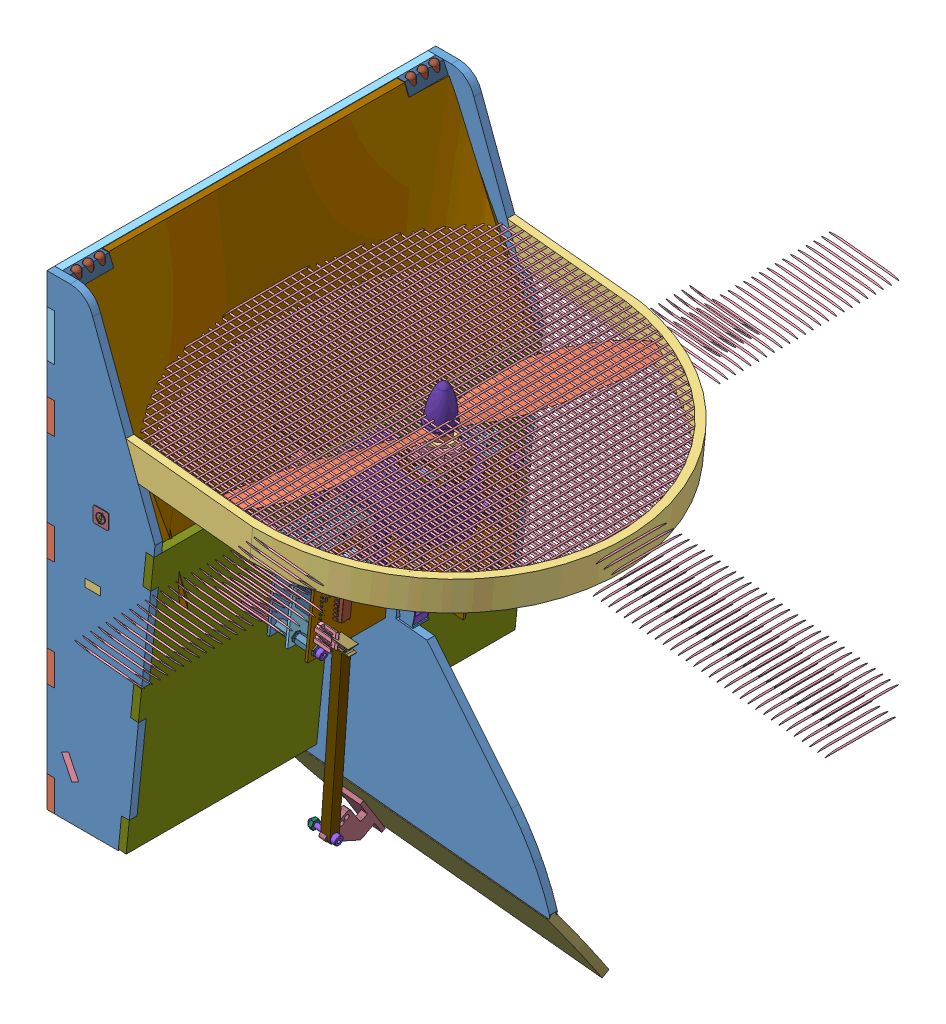
SolidWorks assembly AssTotaleSimu6, configuration Défaut. Lengths in mm.
Overall size (253.25 382.9 251.6).
1779 component instances, 238 part files, 11 mates.
Components (placement in the parent):
- AssStructSimu-1: AssStructSimu [Défaut] at (-125.7658 -1.8483 624.6548) x (1 0 0) z (0 0 -1) size (253.25 324.59 251.6)
  - AssBase-1: AssBase [Défaut] at (36.5482 -71.0398 34.0612) size (86.08 302.3 251.6)
    - AssD-1: AssD [Défaut] at (39.0992 31.0201 8.5) size (69.5 300 22)
      - P1-1: P1 [Défaut] at (-95.5819 194.6656 377.5) size (69.5 300 5)
      - P5-1: P5 [Défaut] at (-100.5819 -35.3344 360.5) x (0 1 0) z (1 0 0) size (230 22 5)
    - AssG-1: AssG [Défaut] at (39.0992 31.0201 -236.5) size (69.5 300 22)
      - P1-1: P1 [Défaut] at (-95.5819 194.6656 377.5) size (69.5 300 5)
      - P5-1: P5 [Défaut] at (-95.5819 -35.3344 399.5) x (0 1 0) z (-1 0 0) size (230 22 5)
    - P7-1: P7 [Défaut] at (-1.4828 89.6857 370.5) x (0 0 -1) z (0 -1 0) size (250 54.5 5)
    - P4-1: P4 [Défaut] at (-63.2363 165.9323 386) x (0 0 -1) z (0.898794 -0.438371 0) size (250 60.5 66.27)
    - P3-1: P3 [Défaut] at (-56.4828 -74.3143 146) x (0 0 1) z (-1 0 0) size (250 70 5)
    - P4b-1: P4b [Défaut] at (-58.7423 163.7404 190) x (0 0 1) z (0.438371 0.898794 0) size (152 56 2)
    - battery-1: battery [Défaut] at (-39.0156 204.1861 197.5) x (0 0 1) z (0.898794 -0.438371 0) size (137 43 30)
    - socket head cap screw 4762_din-1: socket head cap screw 4762_din [EN ISO 4762 M3 x 10 - 10N] at (-27.7008 145.2627 193) x (0.438371 0.898794 0) z (0 0 -1) size (13 5.5 5.5)
    - socket head cap screw 4762_din-2: socket head cap screw 4762_din [EN ISO 4762 M3 x 10 - 10N] at (-27.7008 145.2627 339) x (0.438371 0.898794 0) z (-0.791285 0.385936 -0.474259) size (13 5.5 5.5)
    - socket head cap screw 4762_din-3: socket head cap screw 4762_din [EN ISO 4762 M3 x 10 - 10N] at (-42.0815 152.2766 339) x (0.438371 0.898794 0) z (-0.001489 0.000726 -0.999999) size (13 5.5 5.5)
    - socket head cap screw 4762_din-4: socket head cap screw 4762_din [EN ISO 4762 M3 x 10 - 10N] at (-42.0815 152.2766 193) x (0.438371 0.898794 0) z (-0.031331 0.015281 -0.999392) size (13 5.5 5.5)
    - P11-1: P11 [Défaut] at (-57.5734 -73.9703 146.7843) x (0.005072 0 0.999987) z (0.006197 0.999981 -0.000031) size (240 65 164)
    - AssPhare-1: AssPhare [Défaut] at (-52.8518 -67.6977 411) x (0 1 0) z (0 0 -1) size (35.8 8 25)
      - piece_led-1: piece_led [Défaut] at (-6.6166 -3.631 25) size (7 8 25)
      - LED 5mm-1: LED 5mm [Valor predeterminado] at (-0.1166 0.369 30) x (0 0 1) z (-1 0 0) size (10.06 6 40.8)
      - LED 5mm-2: LED 5mm [Valor predeterminado] at (-0.1166 0.369 37.5) x (0 0 1) z (-1 0 0) size (10.06 6 40.8)
      - LED 5mm-3: LED 5mm [Valor predeterminado] at (-0.1166 0.369 45) x (0 0 1) z (-1 0 0) size (10.06 6 40.8)
    - AssPhare-2: AssPhare [Défaut] at (-52.8518 -67.6977 196) x (0 1 0) z (0 0 -1) size (35.8 8 25)
      - piece_led-1: piece_led [Défaut] at (-6.6166 -3.631 25) size (7 8 25)
      - LED 5mm-1: LED 5mm [Valor predeterminado] at (-0.1166 0.369 30) x (0 0 1) z (-1 0 0) size (10.06 6 40.8)
      - LED 5mm-2: LED 5mm [Valor predeterminado] at (-0.1166 0.369 37.5) x (0 0 1) z (-1 0 0) size (10.06 6 40.8)
      - LED 5mm-3: LED 5mm [Valor predeterminado] at (-0.1166 0.369 45) x (0 0 1) z (-1 0 0) size (10.06 6 40.8)
    - AssLogo-1: AssLogo [Défaut] at (-27.8835 45.1673 148.1054) x (-1 0 0) z (0 0 -1) size (10 10 0.8)
      - logo1-1: logo1 [Défaut] at (-6.5271 -4.4734 6.5054) size (5.8 7.71 0.4)
      - logo2-1: logo2 [Défaut] at (-6.4007 -4.4815 7.1054) size (10 10 0.4)
    - AssLogo-2: AssLogo [Défaut] at (-25.082 45.1673 383.8946) size (10 10 0.8)
      - logo1-1: logo1 [Défaut] at (-6.5271 -4.4734 6.5054) size (5.8 7.71 0.4)
      - logo2-1: logo2 [Défaut] at (-6.4007 -4.4815 7.1054) size (10 10 0.4)
    - support2-1: support2 [Défaut] at (-61.5648 191.7124 276) x (-0.017452 -0.999848 0) z (0.999848 -0.017452 0) size (75 20 10)
    - socket head cap screw 4762_din-5: socket head cap screw 4762_din [EN ISO 4762 M3 x 5 - 5N] at (-61.652 186.7132 269.3333) x (0.999848 -0.017452 0) z (-0.002158 -0.123615 0.992328) size (8 5.5 5.5)
    - socket head cap screw 4762_din-6: socket head cap screw 4762_din [EN ISO 4762 M3 x 5 - 5N] at (-61.652 186.7132 262.6667) x (0.999848 -0.017452 0) z (0 0 1) size (8 5.5 5.5)
    - socket head cap screw 4762_din-7: socket head cap screw 4762_din [EN ISO 4762 M3 x 25 - 18N] at (-55.2963 121.0922 253) x (0 0 1) z (-1 0 0) size (28 5.5 5.5)
    - hex nut style 1 gradeab_din-1: hex nut style 1 gradeab_din [Hexagon Nut ISO 4032 - M3 - W - N] at (-55.2963 121.0922 276) x (-0.923728 -0.383049 0) z (0 0 -1) size (5.5 6.35 2.4)
  - AssToitMot-1: AssToitMot [Défaut] at (-168.5238 43.6961 238.494) x (0 0 -1) z (0.9948 0.101852 0) size (250 207.5 205)
    - AssToit-1: AssToit [Défaut] at (-23.0702 -16.5789 -3.7148) size (250 207.5 205)
      - P8-1: P8 [Défaut] at (-38.4971 122.5921 203.5) size (250 175 5)
      - P12-1: P12 [Défaut] at (-60.4971 -63.4079 265.5) x (1 0 0) z (0 -1 0) size (44.28 76.64 55)
      - P13-1: P13 [Défaut] at (-35.9971 -52.8579 208.5) x (0 0 1) z (-1 0 0) size (64 15.55 5)
      - P10_2-1: P10_2 [Défaut] at (-35.9971 111.5921 171) x (0 0 1) z (-1 0 0) size (188.5 117.6 5)
    - Parallax-Servo_DUMMY-1: Parallax-Servo_DUMMY [Défaut] at (-61.6002 -51.5207 216.6662) x (1 0 0) z (0 1 0) size (20.07 42.67 55.64)
    - socket head cap screw 4762_din-1: socket head cap screw 4762_din [EN ISO 4762 M2.5 x 5 - 5N] at (-51.9272 -76.4868 259.2852) x (0 -1 0) z (-0.546944 0 0.837169) size (7.5 4.5 4.5)
    - socket head cap screw 4762_din-2: socket head cap screw 4762_din [EN ISO 4762 M2.5 x 5 - 5N] at (-61.5672 -76.4868 268.9252) x (0 -1 0) z (-0.546944 0 0.837169) size (7.5 4.5 4.5)
    - socket head cap screw 4762_din-3: socket head cap screw 4762_din [EN ISO 4762 M2.5 x 5 - 5N] at (-71.2072 -76.4868 259.2852) x (0 -1 0) z (-0.546944 0 0.837169) size (7.5 4.5 4.5)
    - socket head cap screw 4762_din-4: socket head cap screw 4762_din [EN ISO 4762 M2.5 x 5 - 5N] at (-61.5672 -76.4868 249.6452) x (0 -1 0) z (-0.546944 0 0.837169) size (7.5 4.5 4.5)
    - AssPhare-1: AssPhare [Défaut] at (8.4328 83.3966 196.1542) x (0 -1 0) z (1 0 0) size (35.8 8 25)
      - piece_led-1: piece_led [Défaut] at (-6.6166 -3.631 25) size (7 8 25)
      - LED 5mm-1: LED 5mm [Valor predeterminado] at (-0.1166 0.369 30) x (0 0 1) z (-1 0 0) size (10.06 6 40.8)
      - LED 5mm-2: LED 5mm [Valor predeterminado] at (-0.1166 0.369 37.5) x (0 0 1) z (-1 0 0) size (10.06 6 40.8)
      - LED 5mm-3: LED 5mm [Valor predeterminado] at (-0.1166 0.369 45) x (0 0 1) z (-1 0 0) size (10.06 6 40.8)
    - AssPhare-2: AssPhare [Défaut] at (-206.5672 83.3966 196.1542) x (0 -1 0) z (1 0 0) size (35.8 8 25)
      - piece_led-1: piece_led [Défaut] at (-6.6166 -3.631 25) size (7 8 25)
      - LED 5mm-1: LED 5mm [Valor predeterminado] at (-0.1166 0.369 30) x (0 0 1) z (-1 0 0) size (10.06 6 40.8)
      - LED 5mm-2: LED 5mm [Valor predeterminado] at (-0.1166 0.369 37.5) x (0 0 1) z (-1 0 0) size (10.06 6 40.8)
      - LED 5mm-3: LED 5mm [Valor predeterminado] at (-0.1166 0.369 45) x (0 0 1) z (-1 0 0) size (10.06 6 40.8)
    - socket head cap screw 4762_din-5: socket head cap screw 4762_din [EN ISO 4762 M3 x 10 - 10N] at (-67.0672 -22.9368 210.2852) x (0 0 -1) z (1 0 0) size (13 5.5 5.5)
    - socket head cap screw 4762_din-6: socket head cap screw 4762_din [EN ISO 4762 M3 x 10 - 10N] at (-56.0672 -72.9868 210.2852) x (0 0 -1) z (1 0 0) size (13 5.5 5.5)
    - socket head cap screw 4762_din-7: socket head cap screw 4762_din [EN ISO 4762 M3 x 10 - 10N] at (-67.0672 -72.9868 210.2852) x (0 0 -1) z (1 0 0) size (13 5.5 5.5)
    - socket head cap screw 4762_din-8: socket head cap screw 4762_din [EN ISO 4762 M3 x 10 - 10N] at (-56.0672 -22.9368 210.2852) x (0 0 -1) z (1 0 0) size (13 5.5 5.5)
    - hex nut style 1 gradeab_din-1: hex nut style 1 gradeab_din [Hexagon Nut ISO 4032 - M3 - W - N] at (-67.0672 -72.9868 197.3852) x (-0.923728 -0.383049 0) z (0 0 -1) size (5.5 6.35 2.4)
    - hex nut style 1 gradeab_din-2: hex nut style 1 gradeab_din [Hexagon Nut ISO 4032 - M3 - W - N] at (-56.0672 -72.9868 199.7852) size (5.5 6.35 2.4)
    - hex nut style 1 gradeab_din-3: hex nut style 1 gradeab_din [Hexagon Nut ISO 4032 - M3 - W - N] at (-67.0672 -22.9368 199.7852) size (5.5 6.35 2.4)
    - hex nut style 1 gradeab_din-4: hex nut style 1 gradeab_din [Hexagon Nut ISO 4032 - M3 - W - N] at (-56.0672 -22.9368 199.7852) size (5.5 6.35 2.4)
  - AssProtec-1: AssProtec [Défaut] at (86.6746 190.4649 284.6351) x (0 0 -1) z (0.101852 -0.9948 0) size (250 237.46 20)
    - protec3c-1: protec3c [Défaut] at (-140.4261 -87.7568 240) size (250 197 20)
    - AssGrillage-1: AssGrillage [Défaut] at (-370.4609 -132.5428 258.3161) x (0 0 -1) z (1 0 0) size (2.02 237.05 250)
      - barreau-1: barreau [Défaut] at (-1.1839 0.254 200) size (1 1 400)
      - barreau-3: barreau [Défaut] at (-1.1839 5.254 200) size (1 1 400)
      - barreau-4: barreau [Défaut] at (-1.1839 10.254 200) size (1 1 400)
      - barreau-5: barreau [Défaut] at (-1.1839 15.254 200) size (1 1 400)
      - barreau-6: barreau [Défaut] at (-1.1839 20.254 200) size (1 1 400)
      - barreau-7: barreau [Défaut] at (-1.1839 25.254 200) size (1 1 400)
      - barreau-8: barreau [Défaut] at (-1.1839 30.254 200) size (1 1 400)
      - barreau-9: barreau [Défaut] at (-1.1839 35.254 200) size (1 1 400)
      - barreau-10: barreau [Défaut] at (-1.1839 40.254 200) size (1 1 400)
      - barreau-11: barreau [Défaut] at (-1.1839 45.254 200) size (1 1 400)
      - barreau-12: barreau [Défaut] at (-1.1839 50.254 200) size (1 1 400)
      - barreau-13: barreau [Défaut] at (-1.1839 55.254 200) size (1 1 400)
      - barreau-14: barreau [Défaut] at (-1.1839 60.254 200) size (1 1 400)
      - barreau-15: barreau [Défaut] at (-1.1839 65.254 200) size (1 1 400)
      - barreau-16: barreau [Défaut] at (-1.1839 70.254 200) size (1 1 400)
      - barreau-17: barreau [Défaut] at (-1.1839 75.254 200) size (1 1 400)
      - barreau-18: barreau [Défaut] at (-1.1839 80.254 200) size (1 1 400)
      - barreau-19: barreau [Défaut] at (-1.1839 85.254 200) size (1 1 400)
      - barreau-20: barreau [Défaut] at (-1.1839 90.254 200) size (1 1 400)
      - barreau-21: barreau [Défaut] at (-1.1839 95.254 200) size (1 1 400)
      - barreau-22: barreau [Défaut] at (-1.1839 100.254 200) size (1 1 400)
      - barreau-23: barreau [Défaut] at (-1.1839 105.254 200) size (1 1 400)
      - barreau-24: barreau [Défaut] at (-1.1839 110.254 200) size (1 1 400)
      - barreau-25: barreau [Défaut] at (-1.1839 115.254 200) size (1 1 400)
      - barreau-26: barreau [Défaut] at (-1.1839 120.254 200) size (1 1 400)
      - barreau-27: barreau [Défaut] at (-1.1839 125.254 200) size (1 1 400)
      - barreau-28: barreau [Défaut] at (-1.1839 130.254 200) size (1 1 400)
      - barreau-29: barreau [Défaut] at (-1.1839 135.254 200) size (1 1 400)
      - barreau-30: barreau [Défaut] at (-1.1839 140.254 200) size (1 1 400)
      - barreau-31: barreau [Défaut] at (-1.1839 145.254 200) size (1 1 400)
      - barreau-32: barreau [Défaut] at (-1.1839 150.254 200) size (1 1 400)
      - barreau-33: barreau [Défaut] at (-1.1839 155.254 200) size (1 1 400)
      - barreau-34: barreau [Défaut] at (-1.1839 160.254 200) size (1 1 400)
      - barreau-35: barreau [Défaut] at (-1.1839 165.254 200) size (1 1 400)
      - barreau-36: barreau [Défaut] at (-1.1839 170.254 200) size (1 1 400)
      - barreau-37: barreau [Défaut] at (-1.1839 175.254 200) size (1 1 400)
      - barreau-38: barreau [Défaut] at (-1.1839 180.254 200) size (1 1 400)
      - barreau-39: barreau [Défaut] at (-1.1839 185.254 200) size (1 1 400)
      - barreau-40: barreau [Défaut] at (-1.1839 190.254 200) size (1 1 400)
      - barreau-41: barreau [Défaut] at (-1.1839 195.254 200) size (1 1 400)
      - barreau-42: barreau [Défaut] at (-0.1839 -1.5314 598.7823) x (0.998922 0 0.04641) z (0 1 0) size (1 1 400)
      - barreau-43: barreau [Défaut] at (-1.1839 200.254 200) size (1 1 400)
      - barreau-44: barreau [Défaut] at (-1.1839 205.254 200) size (1 1 400)
      - barreau-45: barreau [Défaut] at (-1.1839 210.254 200) size (1 1 400)
      - barreau-46: barreau [Défaut] at (-1.1839 215.254 200) size (1 1 400)
      - barreau-47: barreau [Défaut] at (-1.1839 220.254 200) size (1 1 400)
      - barreau-48: barreau [Défaut] at (-1.1839 225.254 200) size (1 1 400)
      - barreau-49: barreau [Défaut] at (-1.1839 230.254 200) size (1 1 400)
      - barreau-50: barreau [Défaut] at (-1.1839 235.254 200) size (1 1 400)
      - barreau-51: barreau [Défaut] at (-1.1839 240.254 200) size (1 1 400)
      - barreau-52: barreau [Défaut] at (-1.1839 245.254 200) size (1 1 400)
      - barreau-53: barreau [Défaut] at (-1.1839 250.254 200) size (1 1 400)
      - barreau-54: barreau [Défaut] at (-1.1839 255.254 200) size (1 1 400)
      - barreau-55: barreau [Défaut] at (-1.1839 260.254 200) size (1 1 400)
      - barreau-56: barreau [Défaut] at (-1.1839 265.254 200) size (1 1 400)
      - barreau-57: barreau [Défaut] at (-1.1839 270.254 200) size (1 1 400)
      - barreau-58: barreau [Défaut] at (-1.1839 275.254 200) size (1 1 400)
      - barreau-59: barreau [Défaut] at (-1.1839 280.254 200) size (1 1 400)
      - barreau-60: barreau [Défaut] at (-1.1839 285.254 200) size (1 1 400)
      - barreau-61: barreau [Défaut] at (-1.1839 290.254 200) size (1 1 400)
      - barreau-62: barreau [Défaut] at (-1.1839 295.254 200) size (1 1 400)
      - barreau-63: barreau [Défaut] at (-1.1839 300.254 200) size (1 1 400)
      - barreau-64: barreau [Défaut] at (-1.1839 305.254 200) size (1 1 400)
      - barreau-65: barreau [Défaut] at (-1.1839 310.254 200) size (1 1 400)
      - barreau-66: barreau [Défaut] at (-1.1839 315.254 200) size (1 1 400)
      - barreau-67: barreau [Défaut] at (-1.1839 320.254 200) size (1 1 400)
      - barreau-68: barreau [Défaut] at (-1.1839 325.254 200) size (1 1 400)
      - barreau-69: barreau [Défaut] at (-1.1839 330.254 200) size (1 1 400)
      - barreau-70: barreau [Défaut] at (-1.1839 335.254 200) size (1 1 400)
      - barreau-71: barreau [Défaut] at (-1.1839 340.254 200) size (1 1 400)
      - barreau-72: barreau [Défaut] at (-1.1839 345.254 200) size (1 1 400)
      - barreau-73: barreau [Défaut] at (-1.1839 350.254 200) size (1 1 400)
      - barreau-74: barreau [Défaut] at (-1.1839 355.254 200) size (1 1 400)
      - barreau-75: barreau [Défaut] at (-1.1839 360.254 200) size (1 1 400)
      - barreau-76: barreau [Défaut] at (-1.1839 365.254 200) size (1 1 400)
      - barreau-77: barreau [Défaut] at (-1.1839 370.254 200) size (1 1 400)
      - barreau-78: barreau [Défaut] at (-1.1839 375.254 200) size (1 1 400)
      - barreau-79: barreau [Défaut] at (-1.1839 380.254 200) size (1 1 400)
      - barreau-80: barreau [Défaut] at (-1.1839 385.254 200) size (1 1 400)
      - barreau-81: barreau [Défaut] at (-1.1839 390.254 200) size (1 1 400)
      - barreau-82: barreau [Défaut] at (-1.1839 395.254 200) size (1 1 400)
      - barreau-136: barreau [Défaut] at (-0.1839 -1.5314 593.7823) x (0.998922 0 0.04641) z (0 1 0) size (1 1 400)
      - barreau-137: barreau [Défaut] at (-0.1839 -1.5314 588.7823) x (0.998922 0 0.04641) z (0 1 0) size (1 1 400)
      - barreau-138: barreau [Défaut] at (-0.1839 -1.5314 583.7823) x (0.998922 0 0.04641) z (0 1 0) size (1 1 400)
      - barreau-139: barreau [Défaut] at (-0.1839 -1.5314 578.7823) x (0.998922 0 0.04641) z (0 1 0) size (1 1 400)
      - barreau-140: barreau [Défaut] at (-0.1839 -1.5314 573.7823) x (0.998922 0 0.04641) z (0 1 0) size (1 1 400)
      - barreau-141: barreau [Défaut] at (-0.1839 -1.5314 568.7823) x (0.998922 0 0.04641) z (0 1 0) size (1 1 400)
      - barreau-142: barreau [Défaut] at (-0.1839 -1.5314 563.7823) x (0.998922 0 0.04641) z (0 1 0) size (1 1 400)
      - barreau-143: barreau [Défaut] at (-0.1839 -1.5314 558.7823) x (0.998922 0 0.04641) z (0 1 0) size (1 1 400)
      - barreau-144: barreau [Défaut] at (-0.1839 -1.5314 553.7823) x (0.998922 0 0.04641) z (0 1 0) size (1 1 400)
      - barreau-145: barreau [Défaut] at (-0.1839 -1.5314 548.7823) x (0.998922 0 0.04641) z (0 1 0) size (1 1 400)
      - barreau-146: barreau [Défaut] at (-0.1839 -1.5314 543.7823) x (0.998922 0 0.04641) z (0 1 0) size (1 1 400)
      - barreau-147: barreau [Défaut] at (-0.1839 -1.5314 538.7823) x (0.998922 0 0.04641) z (0 1 0) size (1 1 400)
      - barreau-148: barreau [Défaut] at (-0.1839 -1.5314 533.7823) x (0.998922 0 0.04641) z (0 1 0) size (1 1 400)
      - barreau-149: barreau [Défaut] at (-0.1839 -1.5314 528.7823) x (0.998922 0 0.04641) z (0 1 0) size (1 1 400)
      - barreau-150: barreau [Défaut] at (-0.1839 -1.5314 523.7823) x (0.998922 0 0.04641) z (0 1 0) size (1 1 400)
      - barreau-151: barreau [Défaut] at (-0.1839 -1.5314 518.7823) x (0.998922 0 0.04641) z (0 1 0) size (1 1 400)
      - barreau-152: barreau [Défaut] at (-0.1839 -1.5314 513.7823) x (0.998922 0 0.04641) z (0 1 0) size (1 1 400)
      - barreau-153: barreau [Défaut] at (-0.1839 -1.5314 508.7823) x (0.998922 0 0.04641) z (0 1 0) size (1 1 400)
      - barreau-154: barreau [Défaut] at (-0.1839 -1.5314 503.7823) x (0.998922 0 0.04641) z (0 1 0) size (1 1 400)
      - barreau-155: barreau [Défaut] at (-0.1839 -1.5314 498.7823) x (0.998922 0 0.04641) z (0 1 0) size (1 1 400)
      - barreau-156: barreau [Défaut] at (-0.1839 -1.5314 493.7823) x (0.998922 0 0.04641) z (0 1 0) size (1 1 400)
      - barreau-157: barreau [Défaut] at (-0.1839 -1.5314 488.7823) x (0.998922 0 0.04641) z (0 1 0) size (1 1 400)
      - barreau-158: barreau [Défaut] at (-0.1839 -1.5314 483.7823) x (0.998922 0 0.04641) z (0 1 0) size (1 1 400)
      - barreau-159: barreau [Défaut] at (-0.1839 -1.5314 478.7823) x (0.998922 0 0.04641) z (0 1 0) size (1 1 400)
      - barreau-160: barreau [Défaut] at (-0.1839 -1.5314 473.7823) x (0.998922 0 0.04641) z (0 1 0) size (1 1 400)
      - barreau-161: barreau [Défaut] at (-0.1839 -1.5314 468.7823) x (0.998922 0 0.04641) z (0 1 0) size (1 1 400)
      - barreau-162: barreau [Défaut] at (-0.1839 -1.5314 463.7823) x (0.998922 0 0.04641) z (0 1 0) size (1 1 400)
      - barreau-163: barreau [Défaut] at (-0.1839 -1.5314 458.7823) x (0.998922 0 0.04641) z (0 1 0) size (1 1 400)
      - barreau-164: barreau [Défaut] at (-0.1839 -1.5314 453.7823) x (0.998922 0 0.04641) z (0 1 0) size (1 1 400)
      - barreau-165: barreau [Défaut] at (-0.1839 -1.5314 448.7823) x (0.998922 0 0.04641) z (0 1 0) size (1 1 400)
      - barreau-166: barreau [Défaut] at (-0.1839 -1.5314 443.7823) x (0.998922 0 0.04641) z (0 1 0) size (1 1 400)
      - barreau-167: barreau [Défaut] at (-0.1839 -1.5314 438.7823) x (0.998922 0 0.04641) z (0 1 0) size (1 1 400)
      - barreau-168: barreau [Défaut] at (-0.1839 -1.5314 433.7823) x (0.998922 0 0.04641) z (0 1 0) size (1 1 400)
      - barreau-169: barreau [Défaut] at (-0.1839 -1.5314 428.7823) x (0.998922 0 0.04641) z (0 1 0) size (1 1 400)
      - barreau-170: barreau [Défaut] at (-0.1839 -1.5314 423.7823) x (0.998922 0 0.04641) z (0 1 0) size (1 1 400)
      - barreau-171: barreau [Défaut] at (-0.1839 -1.5314 418.7823) x (0.998922 0 0.04641) z (0 1 0) size (1 1 400)
      - barreau-172: barreau [Défaut] at (-0.1839 -1.5314 413.7823) x (0.998922 0 0.04641) z (0 1 0) size (1 1 400)
      - barreau-173: barreau [Défaut] at (-0.1839 -1.5314 408.7823) x (0.998922 0 0.04641) z (0 1 0) size (1 1 400)
      - barreau-174: barreau [Défaut] at (-0.1839 -1.5314 403.7823) x (0.998922 0 0.04641) z (0 1 0) size (1 1 400)
      - barreau-175: barreau [Défaut] at (-0.1839 -1.5314 398.7823) x (0.998922 0 0.04641) z (0 1 0) size (1 1 400)
      - barreau-176: barreau [Défaut] at (-0.1839 -1.5314 393.7823) x (0.998922 0 0.04641) z (0 1 0) size (1 1 400)
      - barreau-177: barreau [Défaut] at (-0.1839 -1.5314 388.7823) x (0.998922 0 0.04641) z (0 1 0) size (1 1 400)
      - barreau-178: barreau [Défaut] at (-0.1839 -1.5314 383.7823) x (0.998922 0 0.04641) z (0 1 0) size (1 1 400)
      - barreau-179: barreau [Défaut] at (-0.1839 -1.5314 378.7823) x (0.998922 0 0.04641) z (0 1 0) size (1 1 400)
      - barreau-180: barreau [Défaut] at (-0.1839 -1.5314 373.7823) x (0.998922 0 0.04641) z (0 1 0) size (1 1 400)
      - barreau-181: barreau [Défaut] at (-0.1839 -1.5314 368.7823) x (0.998922 0 0.04641) z (0 1 0) size (1 1 400)
      - barreau-182: barreau [Défaut] at (-0.1839 -1.5314 363.7823) x (0.998922 0 0.04641) z (0 1 0) size (1 1 400)
      - barreau-183: barreau [Défaut] at (-0.1839 -1.5314 358.7823) x (0.998922 0 0.04641) z (0 1 0) size (1 1 400)
      - barreau-184: barreau [Défaut] at (-0.1839 -1.5314 353.7823) x (0.998922 0 0.04641) z (0 1 0) size (1 1 400)
      - barreau-185: barreau [Défaut] at (-0.1839 -1.5314 348.7823) x (0.998922 0 0.04641) z (0 1 0) size (1 1 400)
      - barreau-186: barreau [Défaut] at (-0.1839 -1.5314 343.7823) x (0.998922 0 0.04641) z (0 1 0) size (1 1 400)
      - barreau-187: barreau [Défaut] at (-0.1839 -1.5314 338.7823) x (0.998922 0 0.04641) z (0 1 0) size (1 1 400)
      - barreau-188: barreau [Défaut] at (-0.1839 -1.5314 333.7823) x (0.998922 0 0.04641) z (0 1 0) size (1 1 400)
      - barreau-189: barreau [Défaut] at (-0.1839 -1.5314 328.7823) x (0.998922 0 0.04641) z (0 1 0) size (1 1 400)
      - barreau-190: barreau [Défaut] at (-0.1839 -1.5314 323.7823) x (0.998922 0 0.04641) z (0 1 0) size (1 1 400)
      - barreau-191: barreau [Défaut] at (-0.1839 -1.5314 318.7823) x (0.998922 0 0.04641) z (0 1 0) size (1 1 400)
      - barreau-192: barreau [Défaut] at (-0.1839 -1.5314 313.7823) x (0.998922 0 0.04641) z (0 1 0) size (1 1 400)
      - barreau-193: barreau [Défaut] at (-0.1839 -1.5314 308.7823) x (0.998922 0 0.04641) z (0 1 0) size (1 1 400)
      - barreau-194: barreau [Défaut] at (-0.1839 -1.5314 303.7823) x (0.998922 0 0.04641) z (0 1 0) size (1 1 400)
      - barreau-195: barreau [Défaut] at (-0.1839 -1.5314 298.7823) x (0.998922 0 0.04641) z (0 1 0) size (1 1 400)
      - barreau-196: barreau [Défaut] at (-0.1839 -1.5314 293.7823) x (0.998922 0 0.04641) z (0 1 0) size (1 1 400)
      - barreau-197: barreau [Défaut] at (-0.1839 -1.5314 288.7823) x (0.998922 0 0.04641) z (0 1 0) size (1 1 400)
      - barreau-198: barreau [Défaut] at (-0.1839 -1.5314 283.7823) x (0.998922 0 0.04641) z (0 1 0) size (1 1 400)
      - barreau-199: barreau [Défaut] at (-0.1839 -1.5314 278.7823) x (0.998922 0 0.04641) z (0 1 0) size (1 1 400)
      - barreau-200: barreau [Défaut] at (-0.1839 -1.5314 273.7823) x (0.998922 0 0.04641) z (0 1 0) size (1 1 400)
      - barreau-201: barreau [Défaut] at (-0.1839 -1.5314 268.7823) x (0.998922 0 0.04641) z (0 1 0) size (1 1 400)
      - barreau-202: barreau [Défaut] at (-0.1839 -1.5314 263.7823) x (0.998922 0 0.04641) z (0 1 0) size (1 1 400)
      - barreau-203: barreau [Défaut] at (-0.1839 -1.5314 258.7823) x (0.998922 0 0.04641) z (0 1 0) size (1 1 400)
      - barreau-204: barreau [Défaut] at (-0.1839 -1.5314 253.7823) x (0.998922 0 0.04641) z (0 1 0) size (1 1 400)
      - barreau-205: barreau [Défaut] at (-0.1839 -1.5314 248.7823) x (0.998922 0 0.04641) z (0 1 0) size (1 1 400)
      - barreau-206: barreau [Défaut] at (-0.1839 -1.5314 243.7823) x (0.998922 0 0.04641) z (0 1 0) size (1 1 400)
      - barreau-207: barreau [Défaut] at (-0.1839 -1.5314 238.7823) x (0.998922 0 0.04641) z (0 1 0) size (1 1 400)
      - barreau-208: barreau [Défaut] at (-0.1839 -1.5314 233.7823) x (0.998922 0 0.04641) z (0 1 0) size (1 1 400)
      - barreau-209: barreau [Défaut] at (-0.1839 -1.5314 228.7823) x (0.998922 0 0.04641) z (0 1 0) size (1 1 400)
      - barreau-210: barreau [Défaut] at (-0.1839 -1.5314 223.7823) x (0.998922 0 0.04641) z (0 1 0) size (1 1 400)
      - barreau-211: barreau [Défaut] at (-0.1839 -1.5314 218.7823) x (0.998922 0 0.04641) z (0 1 0) size (1 1 400)
      - barreau-212: barreau [Défaut] at (-0.1839 -1.5314 213.7823) x (0.998922 0 0.04641) z (0 1 0) size (1 1 400)
      - barreau-213: barreau [Défaut] at (-0.1839 -1.5314 208.7823) x (0.998922 0 0.04641) z (0 1 0) size (1 1 400)
      - barreau-214: barreau [Défaut] at (-0.1839 -1.5314 203.7823) x (0.998922 0 0.04641) z (0 1 0) size (1 1 400)
    - AssGrillage-2: AssGrillage [Défaut] at (339.6086 -132.5428 241.6839) x (0 0 1) z (-1 0 0) size (2.02 237.05 250)
      - barreau-1: barreau [Défaut] at (-1.1839 0.254 200) size (1 1 400)
      - barreau-3: barreau [Défaut] at (-1.1839 5.254 200) size (1 1 400)
      - barreau-4: barreau [Défaut] at (-1.1839 10.254 200) size (1 1 400)
      - barreau-5: barreau [Défaut] at (-1.1839 15.254 200) size (1 1 400)
      - barreau-6: barreau [Défaut] at (-1.1839 20.254 200) size (1 1 400)
      - barreau-7: barreau [Défaut] at (-1.1839 25.254 200) size (1 1 400)
      - barreau-8: barreau [Défaut] at (-1.1839 30.254 200) size (1 1 400)
      - barreau-9: barreau [Défaut] at (-1.1839 35.254 200) size (1 1 400)
      - barreau-10: barreau [Défaut] at (-1.1839 40.254 200) size (1 1 400)
      - barreau-11: barreau [Défaut] at (-1.1839 45.254 200) size (1 1 400)
      - barreau-12: barreau [Défaut] at (-1.1839 50.254 200) size (1 1 400)
      - barreau-13: barreau [Défaut] at (-1.1839 55.254 200) size (1 1 400)
      - barreau-14: barreau [Défaut] at (-1.1839 60.254 200) size (1 1 400)
      - barreau-15: barreau [Défaut] at (-1.1839 65.254 200) size (1 1 400)
      - barreau-16: barreau [Défaut] at (-1.1839 70.254 200) size (1 1 400)
      - barreau-17: barreau [Défaut] at (-1.1839 75.254 200) size (1 1 400)
      - barreau-18: barreau [Défaut] at (-1.1839 80.254 200) size (1 1 400)
      - barreau-19: barreau [Défaut] at (-1.1839 85.254 200) size (1 1 400)
      - barreau-20: barreau [Défaut] at (-1.1839 90.254 200) size (1 1 400)
      - barreau-21: barreau [Défaut] at (-1.1839 95.254 200) size (1 1 400)
      - barreau-22: barreau [Défaut] at (-1.1839 100.254 200) size (1 1 400)
      - barreau-23: barreau [Défaut] at (-1.1839 105.254 200) size (1 1 400)
      - barreau-24: barreau [Défaut] at (-1.1839 110.254 200) size (1 1 400)
      - barreau-25: barreau [Défaut] at (-1.1839 115.254 200) size (1 1 400)
      - barreau-26: barreau [Défaut] at (-1.1839 120.254 200) size (1 1 400)
      - barreau-27: barreau [Défaut] at (-1.1839 125.254 200) size (1 1 400)
      - barreau-28: barreau [Défaut] at (-1.1839 130.254 200) size (1 1 400)
      - barreau-29: barreau [Défaut] at (-1.1839 135.254 200) size (1 1 400)
      - barreau-30: barreau [Défaut] at (-1.1839 140.254 200) size (1 1 400)
      - barreau-31: barreau [Défaut] at (-1.1839 145.254 200) size (1 1 400)
      - barreau-32: barreau [Défaut] at (-1.1839 150.254 200) size (1 1 400)
      - barreau-33: barreau [Défaut] at (-1.1839 155.254 200) size (1 1 400)
      - barreau-34: barreau [Défaut] at (-1.1839 160.254 200) size (1 1 400)
      - barreau-35: barreau [Défaut] at (-1.1839 165.254 200) size (1 1 400)
      - barreau-36: barreau [Défaut] at (-1.1839 170.254 200) size (1 1 400)
      - barreau-37: barreau [Défaut] at (-1.1839 175.254 200) size (1 1 400)
      - barreau-38: barreau [Défaut] at (-1.1839 180.254 200) size (1 1 400)
      - barreau-39: barreau [Défaut] at (-1.1839 185.254 200) size (1 1 400)
      - barreau-40: barreau [Défaut] at (-1.1839 190.254 200) size (1 1 400)
      - barreau-41: barreau [Défaut] at (-1.1839 195.254 200) size (1 1 400)
      - barreau-42: barreau [Défaut] at (-0.1839 -1.5314 598.7823) x (0.998922 0 0.04641) z (0 1 0) size (1 1 400)
      - barreau-43: barreau [Défaut] at (-1.1839 200.254 200) size (1 1 400)
      - barreau-44: barreau [Défaut] at (-1.1839 205.254 200) size (1 1 400)
      - barreau-45: barreau [Défaut] at (-1.1839 210.254 200) size (1 1 400)
      - barreau-46: barreau [Défaut] at (-1.1839 215.254 200) size (1 1 400)
      - barreau-47: barreau [Défaut] at (-1.1839 220.254 200) size (1 1 400)
      - barreau-48: barreau [Défaut] at (-1.1839 225.254 200) size (1 1 400)
      - barreau-49: barreau [Défaut] at (-1.1839 230.254 200) size (1 1 400)
      - barreau-50: barreau [Défaut] at (-1.1839 235.254 200) size (1 1 400)
      - barreau-51: barreau [Défaut] at (-1.1839 240.254 200) size (1 1 400)
      - barreau-52: barreau [Défaut] at (-1.1839 245.254 200) size (1 1 400)
      - barreau-53: barreau [Défaut] at (-1.1839 250.254 200) size (1 1 400)
      - barreau-54: barreau [Défaut] at (-1.1839 255.254 200) size (1 1 400)
      - barreau-55: barreau [Défaut] at (-1.1839 260.254 200) size (1 1 400)
      - barreau-56: barreau [Défaut] at (-1.1839 265.254 200) size (1 1 400)
      - barreau-57: barreau [Défaut] at (-1.1839 270.254 200) size (1 1 400)
      - barreau-58: barreau [Défaut] at (-1.1839 275.254 200) size (1 1 400)
      - barreau-59: barreau [Défaut] at (-1.1839 280.254 200) size (1 1 400)
      - barreau-60: barreau [Défaut] at (-1.1839 285.254 200) size (1 1 400)
      - barreau-61: barreau [Défaut] at (-1.1839 290.254 200) size (1 1 400)
      - barreau-62: barreau [Défaut] at (-1.1839 295.254 200) size (1 1 400)
      - barreau-63: barreau [Défaut] at (-1.1839 300.254 200) size (1 1 400)
      - barreau-64: barreau [Défaut] at (-1.1839 305.254 200) size (1 1 400)
      - barreau-65: barreau [Défaut] at (-1.1839 310.254 200) size (1 1 400)
      - barreau-66: barreau [Défaut] at (-1.1839 315.254 200) size (1 1 400)
      - barreau-67: barreau [Défaut] at (-1.1839 320.254 200) size (1 1 400)
      - barreau-68: barreau [Défaut] at (-1.1839 325.254 200) size (1 1 400)
      - barreau-69: barreau [Défaut] at (-1.1839 330.254 200) size (1 1 400)
      - barreau-70: barreau [Défaut] at (-1.1839 335.254 200) size (1 1 400)
      - barreau-71: barreau [Défaut] at (-1.1839 340.254 200) size (1 1 400)
      - barreau-72: barreau [Défaut] at (-1.1839 345.254 200) size (1 1 400)
      - barreau-73: barreau [Défaut] at (-1.1839 350.254 200) size (1 1 400)
      - barreau-74: barreau [Défaut] at (-1.1839 355.254 200) size (1 1 400)
      - barreau-75: barreau [Défaut] at (-1.1839 360.254 200) size (1 1 400)
      - barreau-76: barreau [Défaut] at (-1.1839 365.254 200) size (1 1 400)
      - barreau-77: barreau [Défaut] at (-1.1839 370.254 200) size (1 1 400)
      - barreau-78: barreau [Défaut] at (-1.1839 375.254 200) size (1 1 400)
      - barreau-79: barreau [Défaut] at (-1.1839 380.254 200) size (1 1 400)
      - barreau-80: barreau [Défaut] at (-1.1839 385.254 200) size (1 1 400)
      - barreau-81: barreau [Défaut] at (-1.1839 390.254 200) size (1 1 400)
      - barreau-82: barreau [Défaut] at (-1.1839 395.254 200) size (1 1 400)
      - barreau-136: barreau [Défaut] at (-0.1839 -1.5314 593.7823) x (0.998922 0 0.04641) z (0 1 0) size (1 1 400)
      - barreau-137: barreau [Défaut] at (-0.1839 -1.5314 588.7823) x (0.998922 0 0.04641) z (0 1 0) size (1 1 400)
      - barreau-138: barreau [Défaut] at (-0.1839 -1.5314 583.7823) x (0.998922 0 0.04641) z (0 1 0) size (1 1 400)
      - barreau-139: barreau [Défaut] at (-0.1839 -1.5314 578.7823) x (0.998922 0 0.04641) z (0 1 0) size (1 1 400)
      - barreau-140: barreau [Défaut] at (-0.1839 -1.5314 573.7823) x (0.998922 0 0.04641) z (0 1 0) size (1 1 400)
      - barreau-141: barreau [Défaut] at (-0.1839 -1.5314 568.7823) x (0.998922 0 0.04641) z (0 1 0) size (1 1 400)
      - barreau-142: barreau [Défaut] at (-0.1839 -1.5314 563.7823) x (0.998922 0 0.04641) z (0 1 0) size (1 1 400)
      - barreau-143: barreau [Défaut] at (-0.1839 -1.5314 558.7823) x (0.998922 0 0.04641) z (0 1 0) size (1 1 400)
      - barreau-144: barreau [Défaut] at (-0.1839 -1.5314 553.7823) x (0.998922 0 0.04641) z (0 1 0) size (1 1 400)
      - barreau-145: barreau [Défaut] at (-0.1839 -1.5314 548.7823) x (0.998922 0 0.04641) z (0 1 0) size (1 1 400)
      - barreau-146: barreau [Défaut] at (-0.1839 -1.5314 543.7823) x (0.998922 0 0.04641) z (0 1 0) size (1 1 400)
      - barreau-147: barreau [Défaut] at (-0.1839 -1.5314 538.7823) x (0.998922 0 0.04641) z (0 1 0) size (1 1 400)
      - barreau-148: barreau [Défaut] at (-0.1839 -1.5314 533.7823) x (0.998922 0 0.04641) z (0 1 0) size (1 1 400)
      - barreau-149: barreau [Défaut] at (-0.1839 -1.5314 528.7823) x (0.998922 0 0.04641) z (0 1 0) size (1 1 400)
      - barreau-150: barreau [Défaut] at (-0.1839 -1.5314 523.7823) x (0.998922 0 0.04641) z (0 1 0) size (1 1 400)
      - barreau-151: barreau [Défaut] at (-0.1839 -1.5314 518.7823) x (0.998922 0 0.04641) z (0 1 0) size (1 1 400)
      - barreau-152: barreau [Défaut] at (-0.1839 -1.5314 513.7823) x (0.998922 0 0.04641) z (0 1 0) size (1 1 400)
      - barreau-153: barreau [Défaut] at (-0.1839 -1.5314 508.7823) x (0.998922 0 0.04641) z (0 1 0) size (1 1 400)
      - barreau-154: barreau [Défaut] at (-0.1839 -1.5314 503.7823) x (0.998922 0 0.04641) z (0 1 0) size (1 1 400)
      - barreau-155: barreau [Défaut] at (-0.1839 -1.5314 498.7823) x (0.998922 0 0.04641) z (0 1 0) size (1 1 400)
      - barreau-156: barreau [Défaut] at (-0.1839 -1.5314 493.7823) x (0.998922 0 0.04641) z (0 1 0) size (1 1 400)
      - barreau-157: barreau [Défaut] at (-0.1839 -1.5314 488.7823) x (0.998922 0 0.04641) z (0 1 0) size (1 1 400)
      - barreau-158: barreau [Défaut] at (-0.1839 -1.5314 483.7823) x (0.998922 0 0.04641) z (0 1 0) size (1 1 400)
      - barreau-159: barreau [Défaut] at (-0.1839 -1.5314 478.7823) x (0.998922 0 0.04641) z (0 1 0) size (1 1 400)
      - barreau-160: barreau [Défaut] at (-0.1839 -1.5314 473.7823) x (0.998922 0 0.04641) z (0 1 0) size (1 1 400)
      - barreau-161: barreau [Défaut] at (-0.1839 -1.5314 468.7823) x (0.998922 0 0.04641) z (0 1 0) size (1 1 400)
      - barreau-162: barreau [Défaut] at (-0.1839 -1.5314 463.7823) x (0.998922 0 0.04641) z (0 1 0) size (1 1 400)
      - barreau-163: barreau [Défaut] at (-0.1839 -1.5314 458.7823) x (0.998922 0 0.04641) z (0 1 0) size (1 1 400)
      - barreau-164: barreau [Défaut] at (-0.1839 -1.5314 453.7823) x (0.998922 0 0.04641) z (0 1 0) size (1 1 400)
      - barreau-165: barreau [Défaut] at (-0.1839 -1.5314 448.7823) x (0.998922 0 0.04641) z (0 1 0) size (1 1 400)
      - barreau-166: barreau [Défaut] at (-0.1839 -1.5314 443.7823) x (0.998922 0 0.04641) z (0 1 0) size (1 1 400)
      - barreau-167: barreau [Défaut] at (-0.1839 -1.5314 438.7823) x (0.998922 0 0.04641) z (0 1 0) size (1 1 400)
      - barreau-168: barreau [Défaut] at (-0.1839 -1.5314 433.7823) x (0.998922 0 0.04641) z (0 1 0) size (1 1 400)
      - barreau-169: barreau [Défaut] at (-0.1839 -1.5314 428.7823) x (0.998922 0 0.04641) z (0 1 0) size (1 1 400)
      - barreau-170: barreau [Défaut] at (-0.1839 -1.5314 423.7823) x (0.998922 0 0.04641) z (0 1 0) size (1 1 400)
      - barreau-171: barreau [Défaut] at (-0.1839 -1.5314 418.7823) x (0.998922 0 0.04641) z (0 1 0) size (1 1 400)
      - barreau-172: barreau [Défaut] at (-0.1839 -1.5314 413.7823) x (0.998922 0 0.04641) z (0 1 0) size (1 1 400)
      - barreau-173: barreau [Défaut] at (-0.1839 -1.5314 408.7823) x (0.998922 0 0.04641) z (0 1 0) size (1 1 400)
      - barreau-174: barreau [Défaut] at (-0.1839 -1.5314 403.7823) x (0.998922 0 0.04641) z (0 1 0) size (1 1 400)
      - barreau-175: barreau [Défaut] at (-0.1839 -1.5314 398.7823) x (0.998922 0 0.04641) z (0 1 0) size (1 1 400)
      - barreau-176: barreau [Défaut] at (-0.1839 -1.5314 393.7823) x (0.998922 0 0.04641) z (0 1 0) size (1 1 400)
      - barreau-177: barreau [Défaut] at (-0.1839 -1.5314 388.7823) x (0.998922 0 0.04641) z (0 1 0) size (1 1 400)
      - barreau-178: barreau [Défaut] at (-0.1839 -1.5314 383.7823) x (0.998922 0 0.04641) z (0 1 0) size (1 1 400)
      - barreau-179: barreau [Défaut] at (-0.1839 -1.5314 378.7823) x (0.998922 0 0.04641) z (0 1 0) size (1 1 400)
      - barreau-180: barreau [Défaut] at (-0.1839 -1.5314 373.7823) x (0.998922 0 0.04641) z (0 1 0) size (1 1 400)
      - barreau-181: barreau [Défaut] at (-0.1839 -1.5314 368.7823) x (0.998922 0 0.04641) z (0 1 0) size (1 1 400)
      - barreau-182: barreau [Défaut] at (-0.1839 -1.5314 363.7823) x (0.998922 0 0.04641) z (0 1 0) size (1 1 400)
      - barreau-183: barreau [Défaut] at (-0.1839 -1.5314 358.7823) x (0.998922 0 0.04641) z (0 1 0) size (1 1 400)
      - barreau-184: barreau [Défaut] at (-0.1839 -1.5314 353.7823) x (0.998922 0 0.04641) z (0 1 0) size (1 1 400)
      - barreau-185: barreau [Défaut] at (-0.1839 -1.5314 348.7823) x (0.998922 0 0.04641) z (0 1 0) size (1 1 400)
      - barreau-186: barreau [Défaut] at (-0.1839 -1.5314 343.7823) x (0.998922 0 0.04641) z (0 1 0) size (1 1 400)
      - barreau-187: barreau [Défaut] at (-0.1839 -1.5314 338.7823) x (0.998922 0 0.04641) z (0 1 0) size (1 1 400)
      - barreau-188: barreau [Défaut] at (-0.1839 -1.5314 333.7823) x (0.998922 0 0.04641) z (0 1 0) size (1 1 400)
      - barreau-189: barreau [Défaut] at (-0.1839 -1.5314 328.7823) x (0.998922 0 0.04641) z (0 1 0) size (1 1 400)
      - barreau-190: barreau [Défaut] at (-0.1839 -1.5314 323.7823) x (0.998922 0 0.04641) z (0 1 0) size (1 1 400)
      - barreau-191: barreau [Défaut] at (-0.1839 -1.5314 318.7823) x (0.998922 0 0.04641) z (0 1 0) size (1 1 400)
      - barreau-192: barreau [Défaut] at (-0.1839 -1.5314 313.7823) x (0.998922 0 0.04641) z (0 1 0) size (1 1 400)
      - barreau-193: barreau [Défaut] at (-0.1839 -1.5314 308.7823) x (0.998922 0 0.04641) z (0 1 0) size (1 1 400)
      - barreau-194: barreau [Défaut] at (-0.1839 -1.5314 303.7823) x (0.998922 0 0.04641) z (0 1 0) size (1 1 400)
      - barreau-195: barreau [Défaut] at (-0.1839 -1.5314 298.7823) x (0.998922 0 0.04641) z (0 1 0) size (1 1 400)
      - barreau-196: barreau [Défaut] at (-0.1839 -1.5314 293.7823) x (0.998922 0 0.04641) z (0 1 0) size (1 1 400)
      - barreau-197: barreau [Défaut] at (-0.1839 -1.5314 288.7823) x (0.998922 0 0.04641) z (0 1 0) size (1 1 400)
      - barreau-198: barreau [Défaut] at (-0.1839 -1.5314 283.7823) x (0.998922 0 0.04641) z (0 1 0) size (1 1 400)
      - barreau-199: barreau [Défaut] at (-0.1839 -1.5314 278.7823) x (0.998922 0 0.04641) z (0 1 0) size (1 1 400)
      - barreau-200: barreau [Défaut] at (-0.1839 -1.5314 273.7823) x (0.998922 0 0.04641) z (0 1 0) size (1 1 400)
      - barreau-201: barreau [Défaut] at (-0.1839 -1.5314 268.7823) x (0.998922 0 0.04641) z (0 1 0) size (1 1 400)
      - barreau-202: barreau [Défaut] at (-0.1839 -1.5314 263.7823) x (0.998922 0 0.04641) z (0 1 0) size (1 1 400)
      - barreau-203: barreau [Défaut] at (-0.1839 -1.5314 258.7823) x (0.998922 0 0.04641) z (0 1 0) size (1 1 400)
      - barreau-204: barreau [Défaut] at (-0.1839 -1.5314 253.7823) x (0.998922 0 0.04641) z (0 1 0) size (1 1 400)
      - barreau-205: barreau [Défaut] at (-0.1839 -1.5314 248.7823) x (0.998922 0 0.04641) z (0 1 0) size (1 1 400)
      - barreau-206: barreau [Défaut] at (-0.1839 -1.5314 243.7823) x (0.998922 0 0.04641) z (0 1 0) size (1 1 400)
      - barreau-207: barreau [Défaut] at (-0.1839 -1.5314 238.7823) x (0.998922 0 0.04641) z (0 1 0) size (1 1 400)
